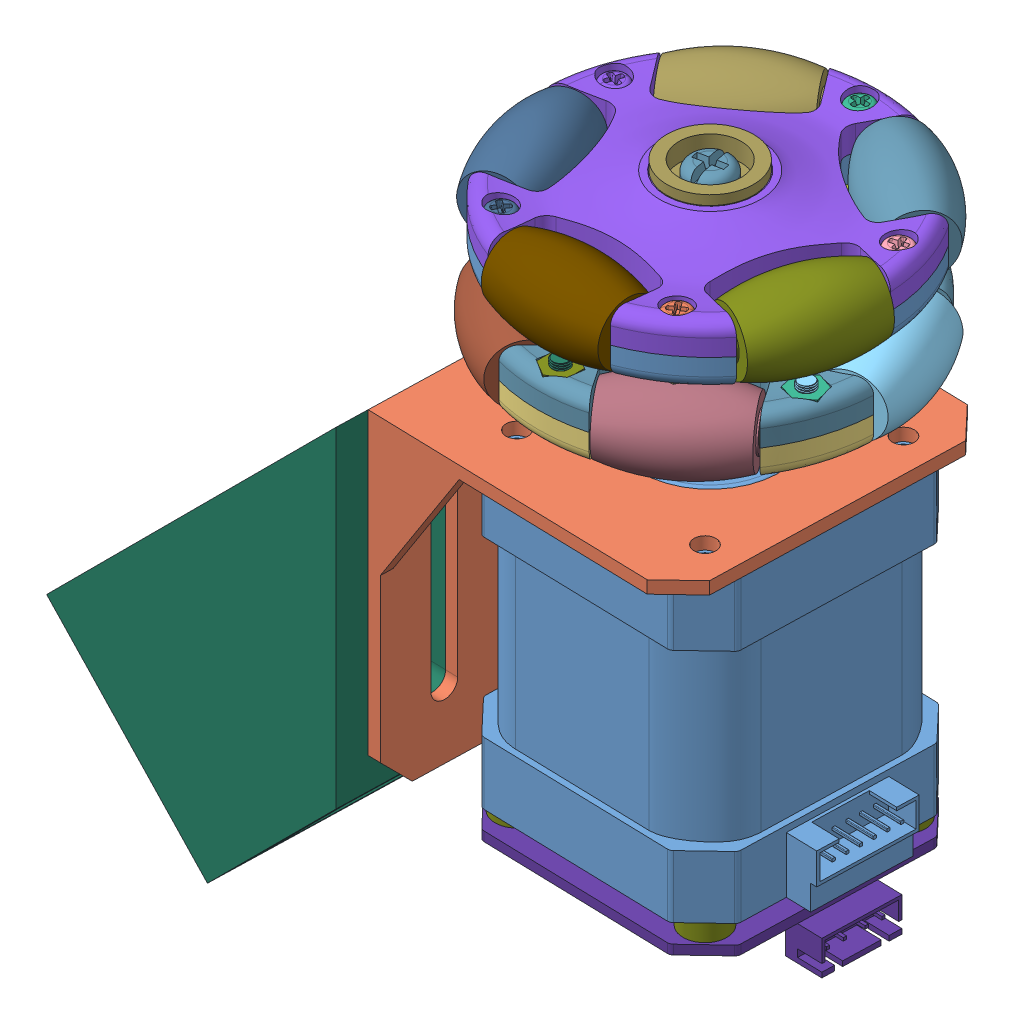
SolidWorks assembly 轮电机装配, configuration 默认. Lengths in mm.
Overall size (112.27 117.96 63.25).
59 component instances, 53 part files, 20 mates.
Components (placement in the parent):
- 42步进电机-1: 42步进电机 [Default] at (113.7797 -206.2562 -45.9286) x (-0.026961 0 0.999636) z (0 1 0) size (42 47 67.8)
- 42步进电机连接件-1: 42步进电机连接件 [默认] at (113.7797 -156.4562 -45.9286) x (0.026961 0 -0.999636) z (-0.999636 0 -0.026961) size (50 53 51)
- 58mm全向轮-2: 58mm全向轮 [默认] at (113.7797 -145.9562 -45.9286) size (67.49 41.74 62.32)
  - 58MMQUANXIANGLUN_DAN-1: 58MMQUANXIANGLUN_DAN [默认] at origin size (67.49 27.49 60.7)
    - DANGPIAN-1-1: DANGPIAN-1 [默认] at origin size (55.41 8.9 53.54)
    - GUNZHOU-1-1: GUNZHOU-1 [默认] at origin size (10.16 3.8 24.74)
    - GUNZI-1-1: GUNZI-1 [默认] at origin size (19.85 20.87 20.84)
    - GUNZHOU_1-1-1: GUNZHOU_1-1 [默认] at origin size (25.2 3.8 3.8)
    - GUNZI_1-1-1: GUNZI_1-1 [默认] at origin size (19.2 13.87 13.87)
    - GUNZHOU_2-1-1: GUNZHOU_2-1 [默认] at origin size (10.16 3.8 24.74)
    - GUNZI_2-1-1: GUNZI_2-1 [默认] at origin size (19.85 20.87 20.84)
    - GUNZHOU_3-1-1: GUNZHOU_3-1 [默认] at origin size (21.86 3.8 16.83)
    - GUNZI_3-1-1: GUNZI_3-1 [默认] at origin size (20.83 27.49 22.24)
    - GUNZHOU_4-1-1: GUNZHOU_4-1 [默认] at origin size (21.86 3.8 16.83)
    - GUNZI_4-1-1: GUNZI_4-1 [默认] at origin size (20.83 27.49 22.24)
    - DANGPIAN_HOU-1-1: DANGPIAN_HOU-1 [默认] at origin size (55.39 8.9 53.54)
    - M3X8-1-1: M3X8-1 [默认] at origin size (4.21 9.65 4.2)
    - M3LUOMU-1-1: M3LUOMU-1 [默认] at origin size (4.9 2 5.66)
    - M3X8_1-1-1: M3X8_1-1 [默认] at origin size (4.2 9.65 4.2)
    - M3LUOMU_1-1-1: M3LUOMU_1-1 [默认] at origin size (5.38 2 5.53)
    - M3X8_2-1-1: M3X8_2-1 [默认] at origin size (4.2 9.65 4.2)
    - M3LUOMU_2-1-1: M3LUOMU_2-1 [默认] at origin size (5.63 2 5.17)
    - M3X8_3-1-1: M3X8_3-1 [默认] at origin size (4.2 9.65 4.2)
    - M3LUOMU_3-1-1: M3LUOMU_3-1 [默认] at origin size (5.63 2 5.17)
    - M3X8_4-1-1: M3X8_4-1 [默认] at origin size (4.2 9.65 4.2)
    - M3LUOMU_4-1-1: M3LUOMU_4-1 [默认] at origin size (5.38 2 5.53)
  - LIANJIEQUAN-1-1: LIANJIEQUAN-1 [默认] at origin size (17 2.5 17)
  - 58MMQUANXIANGLUN_DAN_1-1: 58MMQUANXIANGLUN_DAN_1 [默认] at origin size (67.49 27.49 60.7)
    - DANGPIAN-3-1: DANGPIAN-3 [默认] at origin size (55.41 8.9 53.54)
    - GUNZHOU-3-1: GUNZHOU-3 [默认] at origin size (10.16 3.8 24.74)
    - GUNZI-3-1: GUNZI-3 [默认] at origin size (19.85 20.87 20.84)
    - GUNZHOU_1-3-1: GUNZHOU_1-3 [默认] at origin size (21.86 3.8 16.83)
    - GUNZI_1-3-1: GUNZI_1-3 [默认] at origin size (20.83 27.49 22.24)
    - GUNZHOU_2-3-1: GUNZHOU_2-3 [默认] at origin size (21.86 3.8 16.83)
    - GUNZI_2-3-1: GUNZI_2-3 [默认] at origin size (20.83 27.49 22.24)
    - GUNZHOU_3-3-1: GUNZHOU_3-3 [默认] at origin size (10.16 3.8 24.74)
    - GUNZI_3-3-1: GUNZI_3-3 [默认] at origin size (19.85 20.87 20.84)
    - GUNZHOU_4-3-1: GUNZHOU_4-3 [默认] at origin size (25.2 3.8 3.8)
    - GUNZI_4-3-1: GUNZI_4-3 [默认] at origin size (19.2 13.87 13.87)
    - DANGPIAN_HOU-3-1: DANGPIAN_HOU-3 [默认] at origin size (55.39 8.9 53.54)
    - M3X8-3-1: M3X8-3 [默认] at origin size (4.2 9.65 4.2)
    - M3LUOMU-3-1: M3LUOMU-3 [默认] at origin size (5.63 2 5.17)
    - M3X8_1-3-1: M3X8_1-3 [默认] at origin size (4.2 9.65 4.2)
    - M3LUOMU_1-3-1: M3LUOMU_1-3 [默认] at origin size (5.38 2 5.53)
    - M3X8_2-3-1: M3X8_2-3 [默认] at origin size (4.21 9.65 4.2)
    - M3LUOMU_2-3-1: M3LUOMU_2-3 [默认] at origin size (4.9 2 5.66)
    - M3X8_3-3-1: M3X8_3-3 [默认] at origin size (4.2 9.65 4.2)
    - M3LUOMU_3-3-1: M3LUOMU_3-3 [默认] at origin size (5.38 2 5.53)
    - M3X8_4-3-1: M3X8_4-3 [默认] at origin size (4.2 9.65 4.2)
    - M3LUOMU_4-3-1: M3LUOMU_4-3 [默认] at origin size (5.63 2 5.17)
  - 20170615_LIANZHOUQITAOJIAN4X23-1-1: 20170615_LIANZHOUQITAOJIAN4X23-1 [默认] at origin size (13.9 6 13.9)
  - 20170615_LIANZHOUQI_4X23-1-1: 20170615_LIANZHOUQI_4X23-1 [默认] at origin size (13.9 23 13.9)
  - M4X12-1-1: M4X12-1 [默认] at origin size (6.9 15.15 7.04)
- 底盘连接件-1: 底盘连接件 [默认] at (84.5995 -209.4562 -76.7265) x (-0.026961 0 0.999636) z (0.70685 -0.707107 0.019064) size (60 67.48 37.48)
- 3mm尼龙垫圈高度3mm-1: 3mm尼龙垫圈高度3mm [默认] at (129.692 -209.2562 -61.0051) size (7 3 7)
- 3mm尼龙垫圈高度3mm-2: 3mm尼龙垫圈高度3mm [默认] at (128.8562 -209.2562 -30.0163) size (7 3 7)
- 3mm尼龙垫圈高度3mm-3: 3mm尼龙垫圈高度3mm [默认] at (98.7033 -209.2562 -61.8408) size (7 3 7)
- 3mm尼龙垫圈高度3mm-4: 3mm尼龙垫圈高度3mm [默认] at (97.8675 -209.2562 -30.8521) size (7 3 7)
- 42闭环PCB-1: 42闭环PCB [默认] at (98.7033 -209.2562 -61.8408) x (-1 0 0) z (0 -1 0) size (46.56 42.8 7)
Mates (geometry in assembly coordinates):
- 同心2: concentric anti-aligned: cylinder of 42步进电机-1 through (113.7797 -156.4562 -45.9286) axis (0 -1 0) radius 11; cylinder of 42步进电机连接件-1 through (113.7797 -158.4562 -45.9286) axis (0 1 0) radius 11.05
- 同心3: concentric anti-aligned: cylinder of 42步进电机-1 through (128.8562 -158.4562 -30.0163) axis (0 1 0) radius 1.25; circle of 42步进电机连接件-1
- 同心4: concentric aligned: cylinder of 42步进电机-1 through (98.7033 -158.4562 -61.8408) axis (0 1 0) radius 1.25; cylinder of 42步进电机连接件-1 through (98.7033 -158.4562 -61.8408) axis (0 1 0) radius 1.75
- 重合2: coincident anti-aligned: plane of 42步进电机-1 through (113.7797 -158.4562 -45.9286) normal (0 1 0); plane of 42步进电机连接件-1 through (113.7797 -158.4562 -45.9286) normal (0 -1 0)
- 同心5: concentric aligned: cylinder of 42步进电机-1 through (113.7797 -138.4562 -45.9286) axis (0 -1 0) radius 2.5; cylinder of 58mm全向轮-2/20170615_LIANZHOUQI_4X23-1-1 through (113.7797 -136.4562 -45.9286) axis (0 -1 0) radius 3
- 距离1: distance = 2 mm anti-aligned: plane of 42步进电机-1 through (113.7797 -138.4562 -45.9286) normal (0 1 0); plane of 58mm全向轮-2/20170615_LIANZHOUQI_4X23-1-1 through (116.9488 -136.4562 -42.8585) normal (0 -1 0)
- 同心6: concentric aligned: cylinder of 42步进电机连接件-1 through (83.3862 -168.4562 -31.7429) axis (0.999636 0 0.026961) radius 2.1; cylinder of 底盘连接件-1 through (33.4044 -168.4562 -33.0909) axis (0.999636 0 0.026961) radius 2.1
- 同心8: concentric aligned: cylinder of 42步进电机连接件-1 through (83.3862 -198.4562 -31.7429) axis (0.999636 0 0.026961) radius 2.1; cylinder of 底盘连接件-1 through (33.4044 -198.4562 -33.0909) axis (0.999636 0 0.026961) radius 2.1
- 重合3: coincident anti-aligned: plane of 42步进电机连接件-1 through (83.1166 -209.4562 -21.7465) normal (-0.999636 0 -0.026961); plane of 底盘连接件-1 through (84.4647 -209.4562 -71.7283) normal (0.999636 0 0.026961)
- 同心9: concentric anti-aligned: cylinder of 42步进电机连接件-1 through (129.692 -158.4562 -61.0051) axis (0 1 0) radius 1.75; cylinder of 3mm尼龙垫圈高度3mm-1 through (129.692 -206.2562 -61.0051) axis (0 -1 0) radius 1.5
- 重合4: coincident anti-aligned: plane of 42步进电机-1 through (113.7797 -206.2562 -45.9286) normal (0 -1 0); plane of 3mm尼龙垫圈高度3mm-1 through (129.692 -206.2562 -61.0051) normal (0 1 0)
- 同心10: concentric anti-aligned: circle of 42步进电机连接件-1; circle of 3mm尼龙垫圈高度3mm-2
- 重合5: coincident anti-aligned: plane of 42步进电机-1 through (113.7797 -206.2562 -45.9286) normal (0 -1 0); plane of 3mm尼龙垫圈高度3mm-2 through (128.8562 -206.2562 -30.0163) normal (0 1 0)
- 同心11: concentric anti-aligned: circle of 42步进电机连接件-1; circle of 3mm尼龙垫圈高度3mm-3
- 重合6: coincident anti-aligned: plane of 42步进电机-1 through (113.7797 -206.2562 -45.9286) normal (0 -1 0); plane of 3mm尼龙垫圈高度3mm-3 through (98.7033 -206.2562 -61.8408) normal (0 1 0)
- 同心12: concentric anti-aligned: cylinder of 42步进电机连接件-1 through (97.8675 -158.4562 -30.8521) axis (0 1 0) radius 1.75; cylinder of 3mm尼龙垫圈高度3mm-4 through (97.8675 -206.2562 -30.8521) axis (0 -1 0) radius 1.5
- 重合7: coincident anti-aligned: plane of 42步进电机-1 through (113.7797 -206.2562 -45.9286) normal (0 -1 0); plane of 3mm尼龙垫圈高度3mm-4 through (97.8675 -206.2562 -30.8521) normal (0 1 0)
- 同心13: concentric anti-aligned: cylinder of 3mm尼龙垫圈高度3mm-1 through (129.692 -206.2562 -61.0051) axis (0 -1 0) radius 1.5; cylinder of 42闭环PCB-1 through (129.692 -210.7562 -61.0051) axis (0 1 0) radius 1.5
- 同心14: concentric anti-aligned: cylinder of 3mm尼龙垫圈高度3mm-4 through (97.8675 -206.2562 -30.8521) axis (0 -1 0) radius 1.5; cylinder of 42闭环PCB-1 through (97.8675 -210.7562 -30.8521) axis (0 1 0) radius 1.5
- 重合11: coincident anti-aligned: plane of 3mm尼龙垫圈高度3mm-1 through (129.692 -209.2562 -61.0051) normal (0 -1 0); plane of 42闭环PCB-1 through (133.3657 -209.2562 -30.3091) normal (0 1 0)
